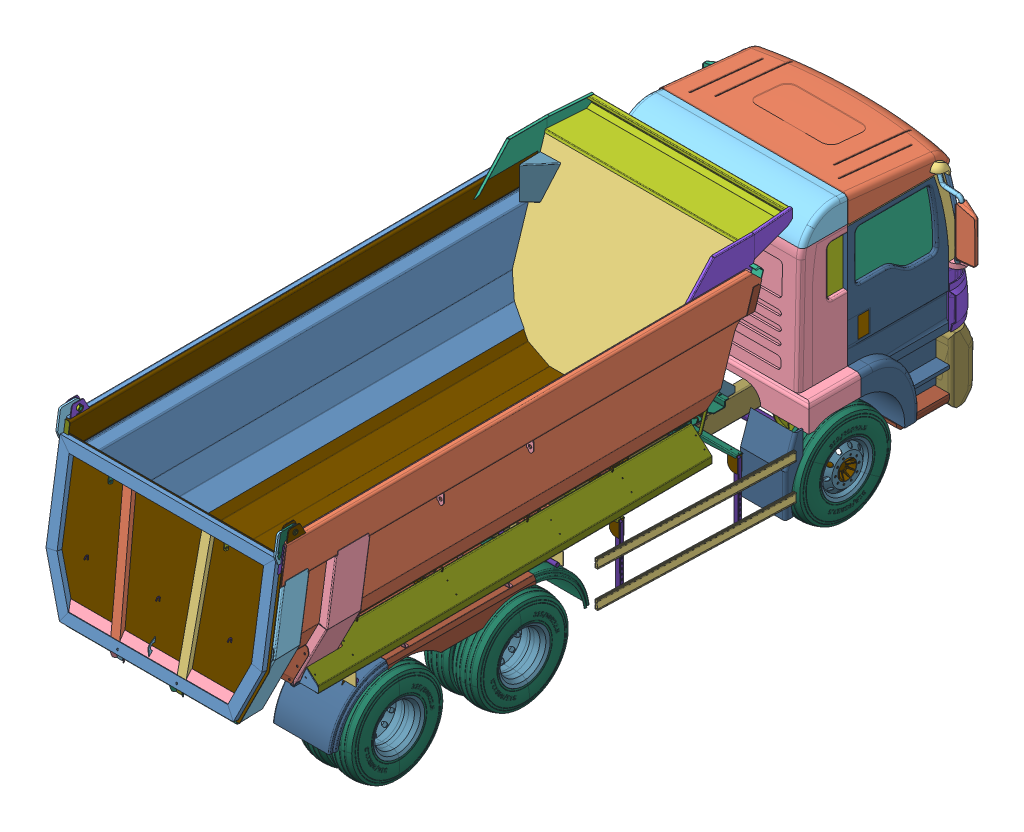
SolidWorks assembly MAN5, configuration Default. Lengths in mm.
Overall size (3197.79 4674.46 9356.54).
475 component instances, 259 part files, 0 mates.
Components (placement in the parent):
- MAN5.IGS-1: MAN5.IGS [Default] at origin size (3197.79 4674.46 9356.54)
  - M5 - Model_004_merkez-2.IGS-1: M5 - Model_004_merkez-2.IGS [Default] at (25.8381 -1.4049 -2.665) size (2122.51 884.45 2018.71)
  - M5 - Model_004_merkez_1-1.IGS-1: M5 - Model_004_merkez_1-1.IGS [Default] at (25.8381 -1.4049 -2.665) size (3165.06 2000 3165.08)
  - M5 - Model_004_merkez_2-1.IGS-1: M5 - Model_004_merkez_2-1.IGS [Default] at (25.8381 -1.4049 -2.665) size (2649.19 3081.51 2336.41)
  - M5 - Model_004_merkez_3-1.IGS-1: M5 - Model_004_merkez_3-1.IGS [Default] at (25.8381 -1.4049 -2.665) size (2847.79 2852 2554.04)
  - M5 - Model_004_merkez_4-1.IGS-1: M5 - Model_004_merkez_4-1.IGS [Default] at (25.8381 -1.4049 -2.665) size (2111.24 616.09 2554.04)
  - M5 - Model_004_merkez_5-1.IGS-1: M5 - Model_004_merkez_5-1.IGS [Default] at (25.8381 -1.4049 -2.665) size (2368.84 1580.76 2801.47)
  - M5 - Model_004_merkez_6-1.IGS-1: M5 - Model_004_merkez_6-1.IGS [Default] at (25.8381 -1.4049 -2.665) size (2552.55 2552.55 2000.01)
  - M5 - Model_004_merkez_7-1.IGS-1: M5 - Model_004_merkez_7-1.IGS [Default] at (25.8381 -1.4049 -2.665) size (2439.28 1485.99 2100.01)
  - M5 - Model_004_merkez_8-1.IGS-1: M5 - Model_004_merkez_8-1.IGS [Default] at (25.8381 -1.4049 -2.665) size (2327.66 2100.01 2220.53)
  - M5 - Model_004_merkez_9-1.IGS-1: M5 - Model_004_merkez_9-1.IGS [Default] at (25.8381 -1.4049 -2.665) size (2931.19 3824.29 2851.69)
  - M5 - Model_004_merkez_10-1.IGS-1: M5 - Model_004_merkez_10-1.IGS [Default] at (25.8381 -1.4049 -2.665) size (2794.82 2200.84 2794.82)
  - M5 - Model_004_merkez_11-1.IGS-1: M5 - Model_004_merkez_11-1.IGS [Default] at (25.8381 -1.4049 -2.665) size (2288.92 905.56 2328.97)
  - M5 - Model_004_Basit_Travers.IGS-1: M5 - Model_004_Basit_Travers.IGS [Default] at (25.8381 1209.558 5190) x (-1 0 0) z (0 0 1) size (746.01 216.01 158.97)
  - M5 - Model_004_Basit_Travers.IGS-2: M5 - Model_004_Basit_Travers.IGS [Default] at (25.8381 1209.558 6590) x (-1 0 0) z (0 0 1) size (746.01 216.01 158.97)
  - M5 - Model_004_Basit_Travers.IGS-3: M5 - Model_004_Basit_Travers.IGS [Default] at (25.8381 1209.558 7350) x (-1 0 0) z (0 0 1) size (746.01 216.01 158.97)
  - M5 - Jant.IGS-1: M5 - Jant.IGS [Default] at (-1015.7235 719.558 1500) size (315.94 575.22 575.22)
  - M5 - Jant.IGS-2: M5 - Jant.IGS [Default] at (1067.3996 719.558 1500) x (-1 0 0) z (0 -0.822188 0.569216) size (315.94 575.22 575.22)
  - M5 - Jant.IGS-3: M5 - Jant.IGS [Default] at (1068.3381 719.558 5100) x (1 0 0) z (0 -0.123259 0.992375) size (315.94 575.22 575.22)
  - M5 - Jant.IGS-4: M5 - Jant.IGS [Default] at (751.4612 719.558 6500) x (-1 0 0) z (0 -0.924225 -0.381849) size (315.94 575.22 575.22)
  - M5 - Jant.IGS-5: M5 - Jant.IGS [Default] at (1068.3381 719.558 6500) size (315.94 575.22 575.22)
  - M5 - Jant.IGS-6: M5 - Jant.IGS [Default] at (751.4612 719.558 5100) x (-1 0 0) z (0 -0.924225 -0.381849) size (315.94 575.22 575.22)
  - M5 - Jant.IGS-7: M5 - Jant.IGS [Default] at (-699.7851 719.558 6500) x (1 0 0) z (0 0.290359 0.956918) size (315.94 575.22 575.22)
  - M5 - Jant.IGS-8: M5 - Jant.IGS [Default] at (-699.7851 719.558 5100) x (1 0 0) z (0 -0.152801 0.988257) size (315.94 575.22 575.22)
  - M5 - Jant.IGS-9: M5 - Jant.IGS [Default] at (-1016.6619 719.558 6500) x (-1 0 0) z (0 -0.924225 -0.381849) size (315.94 575.22 575.22)
  - M5 - Jant.IGS-10: M5 - Jant.IGS [Default] at (-1016.6619 719.558 5100) x (-1 0 0) z (0 -0.924225 -0.381849) size (315.94 575.22 575.22)
  - M5 - Lastik.IGS-1: M5 - Lastik.IGS [Default] at (-1015.7235 719.558 1500) size (336.85 2135.49 1069.79)
  - M5 - Lastik.IGS-2: M5 - Lastik.IGS [Default] at (1067.3996 719.558 1500) x (-1 0 0) z (0 -0.822188 0.569216) size (336.85 2135.49 1069.79)
  - M5 - Lastik.IGS-3: M5 - Lastik.IGS [Default] at (1068.3381 719.558 5100) x (1 0 0) z (0 -0.123259 0.992375) size (336.85 2135.49 1069.79)
  - M5 - Lastik.IGS-4: M5 - Lastik.IGS [Default] at (751.4612 719.558 6500) x (-1 0 0) z (0 -0.924225 -0.381849) size (336.85 2135.49 1069.79)
  - M5 - Lastik.IGS-5: M5 - Lastik.IGS [Default] at (1068.3381 719.558 6500) size (336.85 2135.49 1069.79)
  - M5 - Lastik.IGS-6: M5 - Lastik.IGS [Default] at (751.4612 719.558 5100) x (-1 0 0) z (0 -0.924225 -0.381849) size (336.85 2135.49 1069.79)
  - M5 - Lastik.IGS-7: M5 - Lastik.IGS [Default] at (-699.7851 719.558 6500) x (1 0 0) z (0 0.290359 0.956918) size (336.85 2135.49 1069.79)
  - M5 - Lastik.IGS-8: M5 - Lastik.IGS [Default] at (-699.7851 719.558 5100) x (1 0 0) z (0 -0.152801 0.988257) size (336.85 2135.49 1069.79)
  - M5 - Lastik.IGS-9: M5 - Lastik.IGS [Default] at (-1016.6619 719.558 6500) x (-1 0 0) z (0 -0.924225 -0.381849) size (336.85 2135.49 1069.79)
  - M5 - Lastik.IGS-10: M5 - Lastik.IGS [Default] at (-1016.6619 719.558 5100) x (-1 0 0) z (0 -0.924225 -0.381849) size (336.85 2135.49 1069.79)
  - M5 - Model_004_1.03.IGS-1: M5 - Model_004_1.03.IGS [Default] at (496.0081 1329.558 1500) size (213.27 711.93 203.27)
  - M5 - Model_004_1.03.IGS-2: M5 - Model_004_1.03.IGS [Default] at (406.8381 1329.558 5100) size (213.27 711.93 203.27)
  - M5 - Model_004_1.03.IGS-3: M5 - Model_004_1.03.IGS [Default] at (406.8381 1329.558 6500) size (213.27 711.93 203.27)
  - M5 - Model_004_1.03.IGS-4: M5 - Model_004_1.03.IGS [Default] at (-444.3319 1329.558 1500) x (-1 0 0) z (0 0 -1) size (213.27 711.93 203.27)
  - M5 - Model_004_1.03.IGS-5: M5 - Model_004_1.03.IGS [Default] at (-355.1619 1329.558 6500) x (-1 0 0) z (0 0 -1) size (213.27 711.93 203.27)
  - M5 - Model_004_1.03.IGS-6: M5 - Model_004_1.03.IGS [Default] at (-355.1619 1329.558 5100) x (-1 0 0) z (0 0 -1) size (213.27 711.93 203.27)
  - Part1^M5 - Model_004_merkez.IGS-1: Part1^M5 - Model_004_merkez.IGS [Default] at (696.0081 1329.558 1500) x (0 0 1) z (-1 0 0) size (131.52 131.52 1440.35)
  - Part1^M5 - Model_004_merkez.IGS-2: Part1^M5 - Model_004_merkez.IGS [Default] at (606.8381 1137.1075 5544.6937) x (0 -0.729006 0.684507) z (-1 0 0) size (131.52 131.52 1440.35)
  - Part1^M5 - Model_004_merkez.IGS-3: Part1^M5 - Model_004_merkez.IGS [Default] at (606.8381 1329.558 6500) x (0 0 1) z (-1 0 0) size (131.52 131.52 1440.35)
  - M5 - Model_003_kapak.IGS-1: M5 - Model_003_kapak.IGS [Default] at (1155.4107 719.558 1500) x (-1 0 0) z (0 -0.924225 -0.381849) size (532.33 309.66 309.66)
  - M5 - Model_003_kapak.IGS-2: M5 - Model_003_kapak.IGS [Default] at (-1103.7346 719.558 1500) size (532.33 309.66 309.66)
  - M5 - Model_003_kapak_kýs versiyon.IGS-1: M5 - Model_003_kapak_kýs versiyon.IGS [Default] at (839.4723 719.558 5100) x (-1 0 0) z (0 -0.924225 -0.381849) size (372.33 309.66 309.66)
  - M5 - Model_003_kapak_kýs versiyon.IGS-2: M5 - Model_003_kapak_kýs versiyon.IGS [Default] at (839.4723 719.558 6500) x (-1 0 0) z (0 -0.924225 -0.381849) size (372.33 309.66 309.66)
  - M5 - Model_003_kapak_kýs versiyon.IGS-3: M5 - Model_003_kapak_kýs versiyon.IGS [Default] at (-787.7962 719.558 6500) size (372.33 309.66 309.66)
  - M5 - Model_003_kapak_kýs versiyon.IGS-4: M5 - Model_003_kapak_kýs versiyon.IGS [Default] at (-787.7962 719.558 5100) size (372.33 309.66 309.66)
  - M5 - Model_004_Ayna_01.IGS-1: M5 - Model_004_Ayna_01.IGS [Default] at (1315.5156 2792.184 388.6109) x (0.999312 -0.000007 0.037077) z (0.037077 0.003075 -0.999308) size (228.97 548.09 103.41)
  - Part3^M5 - Model_004_merkez.IGS-1: Part3^M5 - Model_004_merkez.IGS [Default] at (1075.8381 -1.4049 -2.665) x (0 0 -1) z (1 0 0) size (200.04 151.37 108.33)
  - Part4^M5 - Model_004_merkez.IGS-1: Part4^M5 - Model_004_merkez.IGS [Default] at (1075.8381 -1.4049 -2.665) x (0 0 -1) z (1 0 0) size (256.02 80.12 234.96)
  - Part5^M5 - Model_004_merkez.IGS-1: Part5^M5 - Model_004_merkez.IGS [Default] x (0 0 -1) z (1 0 0) size (286.14 989.02 273.84)
  - M5 - MirrorModel_004_Ayna_01.IGS-1: M5 - MirrorModel_004_Ayna_01.IGS [Default] at (-1263.8395 2792.184 388.6109) x (-0.999312 -0.000007 0.037077) z (0.037077 -0.003075 0.999308) size (228.97 548.09 103.41)
  - MirrorPart5^M5 - Model_004_merkez.IGS-1: MirrorPart5^M5 - Model_004_merkez.IGS [Default] at (51.6761 0 0) x (0 0 -1) z (1 0 0) size (286.14 989.02 273.84)
  - MirrorPart3^M5 - Model_004_merkez.IGS-1: MirrorPart3^M5 - Model_004_merkez.IGS [Default] at (-1024.1619 -1.4049 -2.665) x (0 0 -1) z (1 0 0) size (200.04 151.37 108.33)
  - MirrorPart4^M5 - Model_004_merkez.IGS-1: MirrorPart4^M5 - Model_004_merkez.IGS [Default] at (-1024.1619 -1.4049 -2.665) x (0 0 -1) z (1 0 0) size (256.02 79.14 234.96)
  - M5 - Model_004_05.1.IGS-1: M5 - Model_004_05.1.IGS [Default] at (725.8381 719.558 1500) size (611.68 805.68 197.44)
  - M5 - MirrorModel_004_05.1.IGS-1: M5 - MirrorModel_004_05.1.IGS [Default] at (-674.1619 719.558 1500) x (-1 0 0) z (0 0 -1) size (585.64 805.68 197.44)
  - M5 - UV_01.IGS-1: M5 - UV_01.IGS [Default] at (496.0081 1084.558 300) x (0 1 0) z (-1 0 0) size (422.38 7050.01 197.67)
  - M5 - MirrorUV_01.IGS-1: M5 - MirrorUV_01.IGS [Default] at (-444.3319 1084.558 300) x (0 1 0) z (-1 0 0) size (444.78 7050.09 197.67)
  - mandUD-Hekimhan Madencilik_ergünler_3028U þase.IGS-1: mandUD-Hekimhan Madencilik_ergünler_3028U þase.IGS [Default] at (392.7634 1487.0473 7350.78) x (-1 0 0) z (0 0 -1) size (169.56 383.29 5326.56)
  - mandUD-Hekimhan Madencilik_ergünler_3028arka kapama sacý.IGS-1: mandUD-Hekimhan Madencilik_ergünler_3028arka kapama sacý.IGS [Default] at (396.8332 1490.0702 7337.1907) x (0 0 -1) z (1 0 0) size (356.26 207.28 742.01)
  - mandUD-Hekimhan Madencilik_ergünler_3028þase u kapama.IGS-1: mandUD-Hekimhan Madencilik_ergünler_3028þase u kapama.IGS [Default] at (392.7634 1559.558 7350.78) x (-1 0 0) z (0 -1 0) size (150.83 4695.8 209.08)
  - mandUD-Hekimhan Madencilik_ergünler_3028sasidik1.IGS-1: mandUD-Hekimhan Madencilik_ergünler_3028sasidik1.IGS [Default] at (-347.1668 715.695 8942.9949) x (0 0 -1) z (1 0 0) size (75.01 195.01 747.46)
  - mandUD-Hekimhan Madencilik_ergünler_3028sasidik2.IGS-1: mandUD-Hekimhan Madencilik_ergünler_3028sasidik2.IGS [Default] at (-347.1668 520.4685 8982.3981) x (0 0 -1) z (1 0 0) size (146.01 201.01 747.67)
  - mandUD-Hekimhan Madencilik_ergünler_3028sasidik3.IGS-1: mandUD-Hekimhan Madencilik_ergünler_3028sasidik3.IGS [Default] at (336.8332 715.695 3391.5651) x (0 0 1) z (-1 0 0) size (75.01 195.01 622.01)
  - mandUD-Hekimhan Madencilik_ergünler_3028sasidik4.IGS-1: mandUD-Hekimhan Madencilik_ergünler_3028sasidik4.IGS [Default] at (336.8332 520.4685 3352.1619) x (0 0 1) z (-1 0 0) size (146.01 201.01 622.01)
  - mandUD-Hekimhan Madencilik_ergünler_3028þasi çapraz profil.IGS-1: mandUD-Hekimhan Madencilik_ergünler_3028þasi çapraz profil.IGS [Default] at (-204.3626 1420.2443 6969.0489) x (-0.953314 0 -0.30198) z (0.30198 0 -0.953314) size (80.01 120.01 1686.75)
  - mandUD-Hekimhan Madencilik_ergünler_3028þasi u kros.IGS-1: mandUD-Hekimhan Madencilik_ergünler_3028þasi u kros.IGS [Default] at (-42.8668 1670.958 4128.78) x (0 -1 0) z (0 0 1) size (120.16 530.17 70.36)
  - mandUD-Hekimhan Madencilik_ergünler_3028þase  U kros bayraðý.IGS-1: mandUD-Hekimhan Madencilik_ergünler_3028þase  U kros bayraðý.IGS [Default] at (-46.11 1523.1332 3876.3101) x (0 0 1) z (0 -1 0) size (280.01 147.1 51.59)
  - mandUD-Hekimhan Madencilik_ergünler_3028þase  U kros bayraðý.IGS-2: mandUD-Hekimhan Madencilik_ergünler_3028þase  U kros bayraðý.IGS [Default] at (-46.11 1386.9828 4451.6039) x (0 0 -1) z (0 1 0) size (280.01 147.1 51.59)
  - mandUD-Hekimhan Madencilik_ergünler_3028þase  U kros bayraðý.IGS-3: mandUD-Hekimhan Madencilik_ergünler_3028þase  U kros bayraðý.IGS [Default] at (97.7764 1523.1332 4451.6039) x (0 0 -1) z (0 -1 0) size (280.01 147.1 51.59)
  - mandUD-Hekimhan Madencilik_ergünler_3028þase  U kros bayraðý.IGS-4: mandUD-Hekimhan Madencilik_ergünler_3028þase  U kros bayraðý.IGS [Default] at (97.7764 1386.9828 3876.3101) x (0 0 1) z (0 1 0) size (280.01 147.1 51.59)
  - mandUD-Hekimhan Madencilik_ergünler_3028þasi çapraz profil - 2.IGS-1: mandUD-Hekimhan Madencilik_ergünler_3028þasi çapraz profil - 2.IGS [Default] at (256.0549 1412.8718 6969.1172) x (0.952909 0 -0.303256) z (-0.303256 0 -0.952909) size (80.01 120.01 829.1)
  - mandUD-Hekimhan Madencilik_ergünler_3028þasi çapraz profil - 2.IGS-2: mandUD-Hekimhan Madencilik_ergünler_3028þasi çapraz profil - 2.IGS [Default] at (-204.3885 1412.8718 5365.4428) x (-0.952909 0 0.303256) z (0.303256 0 0.952909) size (80.01 120.01 829.1)
  - mandUD-Hekimhan Madencilik_ergünler_3028kulak burcu.IGS-1: mandUD-Hekimhan Madencilik_ergünler_3028kulak burcu.IGS [Default] at (316.8332 1405.558 7270.78) x (0 -0.989813 0.142372) z (1 0 0) size (108.01 108.01 130.01)
  - mandUD-Hekimhan Madencilik_ergünler_3028kulak burcu.IGS-2: mandUD-Hekimhan Madencilik_ergünler_3028kulak burcu.IGS [Default] at (-265.1668 1405.558 7270.78) x (0 0.778674 0.627428) z (-1 0 0) size (108.01 108.01 130.01)
  - mandUD-Hekimhan Madencilik_ergünler_3028þase ön destek.IGS-1: mandUD-Hekimhan Madencilik_ergünler_3028þase ön destek.IGS [Default] at (371.9886 1370.1288 7030.78) size (85.01 115.01 50.01)
  - mandUD-Hekimhan Madencilik_ergünler_3028þase ön destek.IGS-2: mandUD-Hekimhan Madencilik_ergünler_3028þase ön destek.IGS [Default] at (-316.5407 1370.1288 7089.2845) x (-1 0 0) z (0 0 -1) size (85.01 115.01 50.01)
  - mandUD-Hekimhan Madencilik_ergünler_3028þase çaprazlarý ön destek.IGS-1: mandUD-Hekimhan Madencilik_ergünler_3028þase çaprazlarý ön destek.IGS [Default] at (193.5996 1306.8258 5540.2078) x (0.211554 0 -0.977366) z (0.977366 0 0.211554) size (416.64 110.68 170.17)
  - mandUD-Hekimhan Madencilik_ergünler_3028þase çaprazlarý ön destek - 2.IGS-1: mandUD-Hekimhan Madencilik_ergünler_3028þase çaprazlarý ön destek - 2.IGS [Default] at (-147.7974 1306.8258 5541.4771) x (-0.211554 0 -0.977366) z (0.977366 0 -0.211554) size (416.01 111.01 160.55)
  - mandUD-Hekimhan Madencilik_ergünler_3028papatya.IGS-1: mandUD-Hekimhan Madencilik_ergünler_3028papatya.IGS [Default] at (-113.8668 1476.558 5953.1898) x (0 0 1) z (0 1 0) size (362.9 205.5 6.61)
  - mandUD-Hekimhan Madencilik_ergünler_3028papatya.IGS-2: mandUD-Hekimhan Madencilik_ergünler_3028papatya.IGS [Default] at (-113.8668 1350.558 5953.1898) x (0 0 1) z (0 1 0) size (362.9 205.5 6.61)
  - mandUD-Hekimhan Madencilik_ergünler_3028papatyanýn kardeþi.IGS-1: mandUD-Hekimhan Madencilik_ergünler_3028papatyanýn kardeþi.IGS [Default] at (398.5197 1476.558 6712.0341) x (-1 0 0) z (0 1 0) size (185.01 135.01 5.01)
  - mandUD-Hekimhan Madencilik_ergünler_3028papatyanýn kardeþi.IGS-2: mandUD-Hekimhan Madencilik_ergünler_3028papatyanýn kardeþi.IGS [Default] at (-346.8532 1481.558 6712.0341) x (1 0 0) z (0 -1 0) size (185.01 135.01 5.01)
  - mandUD-Hekimhan Madencilik_ergünler_3028papatyanýn kardeþi.IGS-3: mandUD-Hekimhan Madencilik_ergünler_3028papatyanýn kardeþi.IGS [Default] at (-346.8532 1476.558 5622.5259) x (1 0 0) z (0 1 0) size (185.01 135.01 5.01)
  - mandUD-Hekimhan Madencilik_ergünler_3028papatyanýn kardeþi.IGS-4: mandUD-Hekimhan Madencilik_ergünler_3028papatyanýn kardeþi.IGS [Default] at (398.5197 1481.558 5622.5259) x (-1 0 0) z (0 -1 0) size (185.01 135.01 5.01)
  - mandUD-Hekimhan Madencilik_Mirrorergünler_3028U þase.IGS-1: mandUD-Hekimhan Madencilik_Mirrorergünler_3028U þase.IGS [Default] at (1081.4086 1487.0473 7350.78) x (-1 0 0) z (0 0 -1) size (169.56 383.29 5326.56)
  - mandUD-Hekimhan Madencilik_Mirrorergünler_3028þase u kapama.IGS-1: mandUD-Hekimhan Madencilik_Mirrorergünler_3028þase u kapama.IGS [Default] at (1081.4086 1559.558 7350.78) x (-1 0 0) z (0 -1 0) size (150.83 4695.8 209.08)
  - mandUD-Hekimhan Madencilik_1yg01.IGS-1: mandUD-Hekimhan Madencilik_1yg01.IGS [Default] at (-532.224 3095.3268 7897.0296) x (0 0 -1) z (1 0 0) size (477.01 68.01 611.95)
  - mandUD-Volvo_kutu_volvo p1.IGS-1: mandUD-Volvo_kutu_volvo p1.IGS [Default] at (539.0044 1536.3511 2735.78) x (-1 0 0) z (0 0 -1) size (856.57 250.29 10.2)
  - mandUD-Volvo_kutu_volvo p3.IGS-1: mandUD-Volvo_kutu_volvo p3.IGS [Default] at (666.3154 1574.9793 2925.78) x (-1 0 0) z (0 0 -1) size (834.54 138.01 210.01)
  - mandUD-Volvo_kutu_CH806.IGS-1: mandUD-Volvo_kutu_CH806.IGS [Default] at (-163.6611 1635.5904 2844.6012) x (0 0 -1) z (0 -1 0) size (220.01 80.01 20.01)
  - mandUD-Volvo_kutu_CH806.IGS-2: mandUD-Volvo_kutu_CH806.IGS [Default] at (215.3275 1635.5904 2796.9588) x (0 0 1) z (0 -1 0) size (220.01 80.01 20.01)
  - mandUD-Volvo_kutu_CH805.IGS-1: mandUD-Volvo_kutu_CH805.IGS [Default] at (-160.9645 1655.5904 2821.6801) x (0 0 -1) z (0 -1 0) size (220.01 80.01 145.87)
  - mandUD-Volvo_kutu_CH805.IGS-2: mandUD-Volvo_kutu_CH805.IGS [Default] at (212.6309 1655.5904 2819.8799) x (0 0 1) z (0 -1 0) size (220.01 80.01 145.87)
  - mandUD-Volvo_kutu_volvo p5.IGS-1: mandUD-Volvo_kutu_volvo p5.IGS [Default] at (539.0044 1536.3511 2915.78) x (-1 0 0) z (0 0 -1) size (856.93 250.24 10.2)
  - mandUD-altbaský iç.IGS-1: mandUD-altbaský iç.IGS [Default] at (538.0211 1531.0172 2905.78) x (-1 0 0) z (0 0 -1) size (55.01 119.92 170.01)
  - mandAynalamaUD-altbaský iç.IGS-1: mandAynalamaUD-altbaský iç.IGS [Default] at (-486.3547 1531.0172 2905.78) size (55.01 119.92 170.01)
  - manpistonaltbaskýüstsacý_k10_1.IGS-1: manpistonaltbaskýüstsacý_k10_1.IGS [Default] at (-487.338 1535.233 2940.78) x (-1 0 0) z (0 0 -1) size (874.15 50.04 240.01)
  - mandUD-yað tanký ayaðý destek.IGS-1: mandUD-yað tanký ayaðý destek.IGS [Default] at (502.0081 1449.0556 2887.7133) x (0 0 -1) z (1 0 0) size (360.59 98.68 48.4)
  - mandUD-yan lamba kablo borusu.IGS-1: mandUD-yan lamba kablo borusu.IGS [Default] at (326.8332 1422.558 5630.78) x (0 0.985161 0.171635) z (1 0 0) size (42.01 42.01 90.01)
  - mandUD-yan lamba kablo borusu.IGS-2: mandUD-yan lamba kablo borusu.IGS [Default] at (326.8332 1422.558 4185.78) x (0 0.985161 0.171635) z (1 0 0) size (42.01 42.01 90.01)
  - mandUD-yan lamba kablo borusu.IGS-3: mandUD-yan lamba kablo borusu.IGS [Default] at (-365.1668 1422.558 5630.78) x (0 0.784857 0.619677) z (1 0 0) size (42.01 42.01 90.01)
  - mandUD-yan lamba kablo borusu.IGS-4: mandUD-yan lamba kablo borusu.IGS [Default] at (-365.1668 1422.558 4185.78) x (0 0.982686 -0.18528) z (1 0 0) size (42.01 42.01 90.01)
  - mandUD-get ön tak.IGS-1: mandUD-get ön tak.IGS [Default] at (1437.8958 1577.558 5399.2827) x (0.077241 0 -0.997012) z (0 1 0) size (312.01 71.6 10.01)
  - mandud-þase arka iç destek 1.IGS-1: mandud-þase arka iç destek 1.IGS [Default] at (-347.1668 1350.558 7210.78) x (0 0 -1) z (1 0 0) size (130.01 115.24 746.24)
  - mandud-þase arka iç destek 2.IGS-1: mandud-þase arka iç destek 2.IGS [Default] at (398.8332 1365.558 7085.78) x (-1 0 0) z (0 0 -1) size (746.01 5.01 120.01)
  - manÞasi flanþ_k8_4.IGS-1: manÞasi flanþ_k8_4.IGS [Default] at (570.3884 1436.6724 2655.78) x (0 1 0) z (0 0 1) size (152.28 80.01 90.01)
  - manÞasi flanþ_k8_4.IGS-2: manÞasi flanþ_k8_4.IGS [Default] at (481.2135 1436.6724 3935.78) x (0 1 0) z (0 0 1) size (152.28 80.01 90.01)
  - manÞasi flanþ_k8_4.IGS-3: manÞasi flanþ_k8_4.IGS [Default] at (-518.7219 1436.6724 2680.78) x (0 1 0) z (0 0 -1) size (152.28 80.01 90.01)
  - manÞasi flanþ_k8_4.IGS-4: manÞasi flanþ_k8_4.IGS [Default] at (-429.5471 1436.6724 4325.78) x (0 1 0) z (0 0 -1) size (152.28 80.01 90.01)
  - ayakflanþ_k8_4.IGS-1: ayakflanþ_k8_4.IGS [Default] at (-532.3416 1439.2233 2635.78) x (0 0 1) z (-1 0 0) size (90.01 120.01 8.01)
  - ayakflanþ_k8_4.IGS-2: ayakflanþ_k8_4.IGS [Default] at (-443.1668 1439.2233 4280.78) x (0 0 1) z (-1 0 0) size (90.01 120.01 8.01)
  - ayakflanþ_k8_4.IGS-3: ayakflanþ_k8_4.IGS [Default] at (584.0081 1439.2233 2700.78) x (0 0 -1) z (1 0 0) size (90.01 120.01 8.01)
  - ayakflanþ_k8_4.IGS-4: ayakflanþ_k8_4.IGS [Default] at (494.8332 1439.2233 3980.78) x (0 0 -1) z (1 0 0) size (90.01 120.01 8.01)
  - Ayak Sacý1_627.IGS-1: Ayak Sacý1_627.IGS [Default] at (-532.3416 1469.2233 2600.78) x (0 0 1) z (-1 0 0) size (70.01 60.01 627.01)
  - Ayak Sacý3_752.IGS-1: Ayak Sacý3_752.IGS [Default] at (-443.1668 1469.2233 4245.78) x (0 0 1) z (-1 0 0) size (70.01 60.01 752.01)
  - Ayak Sacý2_642.IGS-1: Ayak Sacý2_642.IGS [Default] at (584.0081 1469.2233 2735.78) x (0 0 -1) z (1 0 0) size (70.01 60.01 642.01)
  - Ayak Sacý4_692.IGS-1: Ayak Sacý4_692.IGS [Default] at (494.8332 1469.2233 4015.78) x (0 0 -1) z (1 0 0) size (70.01 60.01 692.01)
  - 132özbmut4900zT13124_ozaas_Part2.IGS-1: 132özbmut4900zT13124_ozaas_Part2.IGS [Default] at (1135.5295 734.2233 2765.9092) x (-1 0 0) z (0 1 0) size (50.39 40.39 700.39)
  - 132özbmut4900zT13124_ozaas_Part2.IGS-2: 132özbmut4900zT13124_ozaas_Part2.IGS [Default] at (1096.3547 734.2233 4045.9092) x (-1 0 0) z (0 1 0) size (50.39 40.39 700.39)
  - 132özbmut4900zT13124_ozaas_Part2.IGS-3: 132özbmut4900zT13124_ozaas_Part2.IGS [Default] at (-1068.8631 734.2233 2570.6508) x (1 0 0) z (0 1 0) size (50.39 40.39 700.39)
  - 132özbmut4900zT13124_ozaas_Part2.IGS-4: 132özbmut4900zT13124_ozaas_Part2.IGS [Default] at (-1104.6883 734.2233 4215.6508) x (1 0 0) z (0 1 0) size (50.39 40.39 700.39)
  - 132özbmut4900zT13124_ozaas_Part1.IGS-1: 132özbmut4900zT13124_ozaas_Part1.IGS [Default] at (1226.0081 1357.4626 2719.3959) x (0 -1 0) z (-1 0 0) size (180.01 52.01 110.01)
  - 132özbmut4900zT13124_ozaas_Part1.IGS-2: 132özbmut4900zT13124_ozaas_Part1.IGS [Default] at (1186.8332 1357.4626 3999.3959) x (0 -1 0) z (-1 0 0) size (180.01 52.01 110.01)
  - 132özbmut4900zT13124_ozaas_Part1.IGS-3: 132özbmut4900zT13124_ozaas_Part1.IGS [Default] at (-1159.3416 1357.4626 2617.1641) x (0 -1 0) z (1 0 0) size (180.01 52.01 110.01)
  - 132özbmut4900zT13124_ozaas_Part1.IGS-4: 132özbmut4900zT13124_ozaas_Part1.IGS [Default] at (-1195.1668 1357.4626 4262.1641) x (0 -1 0) z (1 0 0) size (180.01 52.01 110.01)
  - su tanki ayaði.IGS-1: su tanki ayaði.IGS [Default] at (926.4501 1581.4704 4540.78) x (-1 0 0) z (0 0 1) size (530.27 72.36 35.01)
  - Aynalamasu tanki ayaði.IGS-1: Aynalamasu tanki ayaði.IGS [Default] at (926.4501 1581.4704 4280.78) x (-1 0 0) z (0 0 1) size (529.94 72.36 35.01)
  - alüminyumprofil2150.IGS-1: alüminyumprofil2150.IGS [Default] at (1249.1587 734.2233 2121.7251) x (0.999532 0 0.030591) z (-0.030591 0 0.999532) size (30.01 100.01 2150.01)
  - alüminyumprofil2150.IGS-2: alüminyumprofil2150.IGS [Default] at (1249.1587 1134.2233 2121.7251) x (0.999532 0 0.030591) z (-0.030591 0 0.999532) size (30.01 100.01 2150.01)
  - alüminyumprofil2150.IGS-3: alüminyumprofil2150.IGS [Default] at (-1203.1372 734.2233 4400.78) x (-0.999755 0 -0.022151) z (0.022151 0 -0.999755) size (30.01 100.01 2150.01)
  - alüminyumprofil2150.IGS-4: alüminyumprofil2150.IGS [Default] at (-1203.1372 1134.2233 4400.78) x (-0.999755 0 -0.022151) z (0.022151 0 -0.999755) size (30.01 100.01 2150.01)
  - M33360_26280_L no4.IGS-1: M33360_26280_L no4.IGS [Default] at (-5513.4738 997.2018 5090.78) size (110.01 60.01 60.01)
  - M33360_26280_mil no8.IGS-1: M33360_26280_mil no8.IGS [Default] at (-395.1668 1499.8885 5115.2337) x (0 -0.974556 -0.224142) z (-1 0 0) size (40 40 115.01)
  - M33360_26280_parça no6.IGS-1: M33360_26280_parça no6.IGS [Default] at (-6126.2776 997.122 5116.78) size (85.01 60.01 8.01)
  - M33360_26280_L no3.IGS-1: M33360_26280_L no3.IGS [Default] at (-5513.4738 1007.2018 4505.78) size (110.01 60.01 60.01)
  - M33360_26280_parça no7.IGS-1: M33360_26280_parça no7.IGS [Default] at (-6108.3607 1023.5325 4533.78) size (87.79 49.97 4.01)
  - 33360_33360_esnek V üst parça.IGS-1: 33360_33360_esnek V üst parça.IGS [Default] at (8896.3998 1392.558 424260.0548) x (0 0 -1) z (0 1 0) size (225.37 59.4 97.48)
  - 33360_33360_esnek V üst parça.IGS-2: 33360_33360_esnek V üst parça.IGS [Default] at (-23741.8905 1342.558 424563.3705) x (0.077241 0 -0.997012) z (0 1 0) size (225.37 59.4 97.48)
  - 33360_33360_esnek ust ped.IGS-1: 33360_33360_esnek ust ped.IGS [Default] at (504.0081 -6771.8803 -419424.7262) x (0 0 1) z (-1 0 0) size (244.65 109.81 8.25)
  - 33360_33360_esnek ust ped.IGS-2: 33360_33360_esnek ust ped.IGS [Default] at (33057.9085 -6821.8803 -417249.0937) x (-0.077241 0 0.997012) z (-0.997012 0 -0.077241) size (244.65 109.81 8.25)
  - 33360_33360_2li esnke ara parça.IGS-1: 33360_33360_2li esnke ara parça.IGS [Default] at (423131.3662 -7117.2745 2426.6366) x (-1 0 0) z (0 0 -1) size (52.01 78.06 10.01)
  - 33360_33360_2li esnke ara parça.IGS-2: 33360_33360_2li esnke ara parça.IGS [Default] at (421838.3924 -7167.2745 35986.156) x (-0.997012 0 -0.077241) z (0.077241 0 -0.997012) size (52.01 78.06 10.01)
  - 33360_33360_Esnek V alt parça_uzun.IGS-1: 33360_33360_Esnek V alt parça_uzun.IGS [Default] at (-7741.4899 1377.558 -419416.7816) x (0 0 1) z (0 1 0) size (154.96 57.01 82.86)
  - 33360_33360_ESNEK UZUN ALT PED.IGS-1: 33360_33360_ESNEK UZUN ALT PED.IGS [Default] at (504.008 1377.558 -419416.7816) x (0 0 1) z (-1 0 0) size (155.4 123.02 8.3)
  - 33360_pulll.IGS-1: 33360_pulll.IGS [Default] at (532.7834 1374.558 2462.7366) x (0.995495 0 0.09481) z (0 1 0) size (40 76.01 3.01)
  - 33360_pulll.IGS-2: 33360_pulll.IGS [Default] at (531.1834 1402.558 2461.1366) x (0.995495 0 0.09481) z (0 1 0) size (40 76.01 3.01)
  - 33360_pulll.IGS-3: 33360_pulll.IGS [Default] at (531.1834 1445.558 2461.1366) x (-0.473934 0 -0.88056) z (0 1 0) size (40 76.01 3.01)
  - 33360_pulll.IGS-4: 33360_pulll.IGS [Default] at (531.1834 1445.558 2381.1366) x (-0.473934 0 -0.88056) z (0 1 0) size (40 76.01 3.01)
  - 33360_pulll.IGS-5: 33360_pulll.IGS [Default] at (531.1834 1402.558 2381.1366) x (0.995495 0 0.09481) z (0 1 0) size (40 76.01 3.01)
  - 33360_pulll.IGS-6: 33360_pulll.IGS [Default] at (532.7834 1374.558 2382.7366) x (0.995495 0 0.09481) z (0 1 0) size (40 76.01 3.01)
  - 33360_pulll.IGS-7: 33360_pulll.IGS [Default] at (496.0665 1352.558 3378.3048) x (0.995286 0 0.096983) z (0 1 0) size (40 76.01 3.01)
  - 33360_pulll.IGS-8: 33360_pulll.IGS [Default] at (496.0665 1324.558 3378.3048) x (0.95234 0 -0.30504) z (0 1 0) size (40 76.01 3.01)
  - 33360_pulll.IGS-9: 33360_pulll.IGS [Default] at (502.0141 1324.558 3301.5348) x (0.95234 0 -0.30504) z (0 1 0) size (40 76.01 3.01)
  - 33360_pulll.IGS-10: 33360_pulll.IGS [Default] at (502.0141 1352.558 3301.5348) x (0.995286 0 0.096983) z (0 1 0) size (40 76.01 3.01)
  - 33360_pulll.IGS-11: 33360_pulll.IGS [Default] at (496.0665 1395.558 3378.3048) x (-0.404503 0 -0.914537) z (0 1 0) size (40 76.01 3.01)
  - 33360_pulll.IGS-12: 33360_pulll.IGS [Default] at (502.0141 1395.558 3301.5348) x (-0.404503 0 -0.914537) z (0 1 0) size (40 76.01 3.01)
  - 33360_23658911.IGS-1: 33360_23658911.IGS [Default] at (531.1834 1363.808 2461.1366) x (0 1 0) z (-0.844065 0 0.536241) size (111.08 30.41 27.75)
  - 33360_23658911.IGS-2: 33360_23658911.IGS [Default] at (531.1834 1363.808 2381.1366) x (0 1 0) z (-0.844065 0 0.536241) size (111.08 30.41 27.75)
  - 33360_23658911.IGS-3: 33360_23658911.IGS [Default] at (496.0665 1313.808 3378.3048) x (0 1 0) z (0.505108 0 -0.863056) size (111.08 30.41 27.75)
  - 33360_23658911.IGS-4: 33360_23658911.IGS [Default] at (502.0141 1313.808 3301.5348) x (0 1 0) z (0.505108 0 -0.863056) size (111.08 30.41 27.75)
  - 33360_23658911.IGS-5: 33360_23658911.IGS [Default] at (-479.517 1363.808 2461.1366) x (0 1 0) z (-0.844065 0 -0.536241) size (111.08 30.41 27.75)
  - 33360_23658911.IGS-6: 33360_23658911.IGS [Default] at (-479.5171 1363.808 2381.1365) x (0 1 0) z (-0.844065 0 -0.536241) size (111.08 30.41 27.75)
  - 33360_23658911.IGS-7: 33360_23658911.IGS [Default] at (-444.4001 1313.808 3378.3048) x (0 1 0) z (0.505108 0 0.863056) size (111.08 30.41 27.75)
  - 33360_23658911.IGS-8: 33360_23658911.IGS [Default] at (-450.3476 1313.808 3301.5349) x (0 1 0) z (0.505108 0 0.863056) size (111.08 30.41 27.75)
  - 33360_esnek baglanti poliuretan takoz.IGS-1: 33360_esnek baglanti poliuretan takoz.IGS [Default] at (531.1834 1445.558 2461.1366) x (-0.305771 0 -0.952105) z (-0.952105 0 0.305771) size (40.39 40.39 40.78)
  - 33360_esnek baglanti poliuretan takoz.IGS-2: 33360_esnek baglanti poliuretan takoz.IGS [Default] at (531.1834 1445.558 2381.1366) x (-0.305771 0 -0.952105) z (-0.952105 0 0.305771) size (40.39 40.39 40.78)
  - 33360_HEX NUT - ISO 8673 - M16 X 1.5.IGS-1: 33360_HEX NUT - ISO 8673 - M16 X 1.5.IGS [Default] at (531.1834 1463.358 2461.1366) x (0 -1 0) z (-0.270173 0 0.962812) size (15.03 27.75 27.75)
  - 33360_HEX NUT - ISO 8673 - M16 X 1.5.IGS-2: 33360_HEX NUT - ISO 8673 - M16 X 1.5.IGS [Default] at (531.1834 1463.358 2381.1366) x (0 -1 0) z (-0.270173 0 0.962812) size (15.03 27.75 27.75)
  - 33360_HEX NUT - ISO 8673 - M16 X 1.5.IGS-3: 33360_HEX NUT - ISO 8673 - M16 X 1.5.IGS [Default] at (496.0665 1413.358 3378.3048) x (0 -1 0) z (0.336021 0 0.941854) size (15.03 27.75 27.75)
  - 33360_HEX NUT - ISO 8673 - M16 X 1.5.IGS-4: 33360_HEX NUT - ISO 8673 - M16 X 1.5.IGS [Default] at (502.0141 1413.358 3301.5348) x (0 -1 0) z (0.336021 0 0.941854) size (15.03 27.75 27.75)
  - 33360_MS 008.IGS-1: 33360_MS 008.IGS [Default] at (660.9084 1337.558 3134.9181) x (-0.077241 0 0.997012) z (0 -1 0) size (151.51 57.06 58.88)
  - 33360_MS 009.IGS-1: 33360_MS 009.IGS [Default] at (490.7184 1337.558 3121.7331) x (0.077241 0 -0.997012) z (-0.997012 0 -0.077241) size (151.36 58.71 8.01)
  - 33360_burçlu baðlantý burcu.IGS-1: 33360_burçlu baðlantý burcu.IGS [Default] at (496.0665 1355.558 3378.3048) x (-0.984937 0 0.172914) z (0 1 0) size (42 42 40.01)
  - 33360_burçlu baðlantý burcu.IGS-2: 33360_burçlu baðlantý burcu.IGS [Default] at (502.0141 1355.558 3301.5348) x (-0.984937 0 0.172914) z (0 1 0) size (42 42 40.01)
  - 33360_arkamilbaðlantý.IGS-1: 33360_arkamilbaðlantý.IGS [Default] at (416.8332 311.3597 8865.1072) x (0 0 -1) z (1 0 0) size (490.86 251.62 10.56)
  - 33360_KMS 305.IGS-1: 33360_KMS 305.IGS [Default] at (-449.2659 1593.4723 2439.837) x (-1 0 0) z (0 1 0) size (253.31 189.01 92.34)
  - Son_model_3.IGS-1: Son_model_3.IGS [Default] at (416.8332 1272.558 6138.28) x (0 0 -1) z (1 0 0) size (155.01 200.01 10.32)
  - Son_model_3.IGS-2: Son_model_3.IGS [Default] at (416.8332 1272.558 5438.28) x (0 0 -1) z (1 0 0) size (155.01 200.01 10.32)
  - Son_model_3.IGS-3: Son_model_3.IGS [Default] at (416.8332 1272.558 4408.28) x (0 0 -1) z (1 0 0) size (155.01 200.01 10.32)
  - Aynalama33360_33360_esnek V üst parça.IGS-1: Aynalama33360_33360_esnek V üst parça.IGS [Default] at (-8844.7333 1392.558 424260.0548) x (0 0 -1) z (0 -1 0) size (225.37 59.16 97.25)
  - Aynalama33360_33360_esnek V üst parça.IGS-2: Aynalama33360_33360_esnek V üst parça.IGS [Default] at (23793.5569 1342.558 424563.3705) x (-0.077241 0 -0.997012) z (0 -1 0) size (225.37 59.16 97.25)
  - Aynalama33360_33360_esnek ust ped.IGS-1: Aynalama33360_33360_esnek ust ped.IGS [Default] at (-452.3416 -6771.8803 -419424.7262) x (0 0 1) z (-1 0 0) size (244.57 109.9 8.12)
  - Aynalama33360_33360_esnek ust ped.IGS-2: Aynalama33360_33360_esnek ust ped.IGS [Default] at (-33006.242 -6821.8803 -417249.0936) x (0.077241 0 0.997012) z (-0.997012 0 0.077241) size (244.57 109.9 8.12)
  - Aynalama33360_33360_2li esnke ara parça.IGS-1: Aynalama33360_33360_2li esnke ara parça.IGS [Default] at (-423079.6998 -7117.2745 2426.6366) size (52.01 78.06 10.01)
  - Aynalama33360_33360_2li esnke ara parça.IGS-2: Aynalama33360_33360_2li esnke ara parça.IGS [Default] at (-421786.7259 -7167.2745 35986.156) x (0.997012 0 -0.077241) z (0.077241 0 0.997012) size (52.01 78.06 10.01)
  - Aynalama33360_33360_Esnek V alt parça_uzun.IGS-1: Aynalama33360_33360_Esnek V alt parça_uzun.IGS [Default] at (7793.1563 1377.558 -419416.7816) x (0 0 1) z (0 -1 0) size (154.93 57.12 82.73)
  - Aynalama33360_33360_ESNEK UZUN ALT PED.IGS-1: Aynalama33360_33360_ESNEK UZUN ALT PED.IGS [Default] at (-452.3416 1377.558 -419416.7816) x (0 0 1) z (-1 0 0) size (155.59 123.11 8.39)
  - Aynalama33360_pulll.IGS-1: Aynalama33360_pulll.IGS [Default] at (-481.117 1374.558 2462.7366) x (-0.995495 0 0.09481) z (0 -1 0) size (40 76.01 3.01)
  - Aynalama33360_pulll.IGS-2: Aynalama33360_pulll.IGS [Default] at (-479.517 1402.558 2461.1366) x (-0.995495 0 0.09481) z (0 -1 0) size (40 76.01 3.01)
  - Aynalama33360_pulll.IGS-3: Aynalama33360_pulll.IGS [Default] at (-479.517 1445.558 2461.1366) x (0.473934 0 -0.88056) z (0 -1 0) size (40 76.01 3.01)
  - Aynalama33360_pulll.IGS-4: Aynalama33360_pulll.IGS [Default] at (-479.517 1445.558 2381.1366) x (0.473934 0 -0.88056) z (0 -1 0) size (40 76.01 3.01)
  - Aynalama33360_pulll.IGS-5: Aynalama33360_pulll.IGS [Default] at (-479.517 1402.558 2381.1366) x (-0.995495 0 0.09481) z (0 -1 0) size (40 76.01 3.01)
  - Aynalama33360_pulll.IGS-6: Aynalama33360_pulll.IGS [Default] at (-481.117 1374.558 2382.7366) x (-0.995495 0 0.09481) z (0 -1 0) size (40 76.01 3.01)
  - Aynalama33360_pulll.IGS-7: Aynalama33360_pulll.IGS [Default] at (-444.4001 1352.558 3378.3048) x (-0.995286 0 0.096983) z (0 -1 0) size (40 76.01 3.01)
  - Aynalama33360_pulll.IGS-8: Aynalama33360_pulll.IGS [Default] at (-444.4001 1324.558 3378.3048) x (-0.95234 0 -0.30504) z (0 -1 0) size (40 76.01 3.01)
